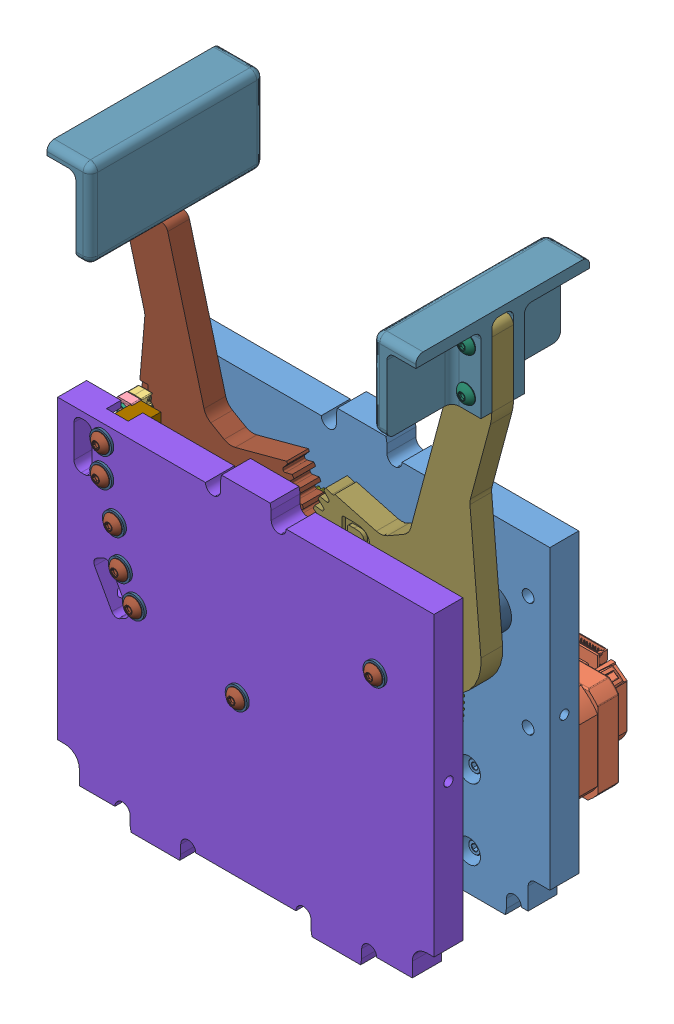
SolidWorks assembly R_ASSY_200_rev3, configuration Default. Lengths in mm. (continued)
Mates (geometry in assembly coordinates): (continued)
- Concentric109: concentric: cylinder of R_203_01_rev4-1 through (-32.103 255.9661 146.893) axis (0 0 1) radius 3.175; cylinder of 91125A453_18-8 SS FEM THRDED ROUND STANDOFF-2 through (-32.103 255.9661 146.893) axis (0 0 -1) radius 3.175
- Width4: width: plane of 91125A453_18-8 SS FEM THRDED ROUND STANDOFF-2 through (-32.103 255.9661 146.893) normal (0 0 1); plane of 91125A453_18-8 SS FEM THRDED ROUND STANDOFF-2 through (-32.103 255.9661 137.368) normal (0 0 -1); plane of R_203_01_rev4-1 through (-14.6848 152.2703 137.368) normal (0 0 -1); plane of R_203_01_rev4-1 through (-14.6848 152.2703 146.893) normal (0 0 1)
- Concentric110: concentric: cylinder of R_203_02_rev4-1 through (117.0334 275.0161 137.368) axis (0 0 -1) radius 3.175; cylinder of 91125A453_18-8 SS FEM THRDED ROUND STANDOFF-4 through (117.0334 275.0161 137.368) axis (0 0 1) radius 3.175
- Width5: width: plane of 91125A453_18-8 SS FEM THRDED ROUND STANDOFF-4 through (117.0334 275.0161 137.368) normal (0 0 -1); plane of 91125A453_18-8 SS FEM THRDED ROUND STANDOFF-4 through (117.0334 275.0161 146.893) normal (0 0 1); plane of R_203_02_rev4-1 through (99.6152 152.2703 146.893) normal (0 0 1); plane of R_203_02_rev4-1 through (99.6152 152.2703 137.368) normal (0 0 -1)
- Concentric111: concentric: cylinder of R_203_02_rev4-1 through (117.0334 255.9661 137.368) axis (0 0 -1) radius 3.175; cylinder of 91125A453_18-8 SS FEM THRDED ROUND STANDOFF-6 through (117.0334 255.9661 137.368) axis (0 0 1) radius 3.175
- Width6: width: plane of 91125A453_18-8 SS FEM THRDED ROUND STANDOFF-6 through (117.0334 255.9661 137.368) normal (0 0 -1); plane of 91125A453_18-8 SS FEM THRDED ROUND STANDOFF-6 through (117.0334 255.9661 146.893) normal (0 0 1); plane of R_203_02_rev4-1 through (99.6152 152.2703 137.368) normal (0 0 -1); plane of R_203_02_rev4-1 through (99.6152 152.2703 146.893) normal (0 0 1)
- Width7: width: plane of R_203_05-1 through (16.7976 249.6161 146.893) normal (0 0 -1); plane of R_203_05-1 through (16.7976 249.6161 137.368) normal (0 0 1); plane of R_203_01_rev4-1 through (-14.6848 152.2703 137.368) normal (0 0 -1); plane of R_203_01_rev4-1 through (-14.6848 152.2703 146.893) normal (0 0 1)
- Concentric112: concentric: cylinder of R_203_01_rev4-1 through (-32.103 275.0161 146.893) axis (0 0 1) radius 3.175; cylinder of R_203_05-1 through (-32.103 275.0161 132.6055) axis (0 0 -1) radius 2.2479
- Concentric113: concentric: cylinder of R_203_01_rev4-1 through (-32.103 255.9661 146.893) axis (0 0 1) radius 3.175; cylinder of R_203_05-1 through (-32.103 255.9661 132.6055) axis (0 0 -1) radius 2.2479
- Concentric114: concentric: cylinder of R_203_05-1 through (-32.103 275.0161 132.6055) axis (0 0 -1) radius 2.2479; cylinder of 92949A192_18-8 SS BUTTON HEAD HEX DRIVE SCREW-19 through (-32.103 275.0161 153.8653) axis (0 0 1) radius 3.9624
- Coincident104: coincident: plane of R_203_05-1 through (18.1551 249.6161 151.6555) normal (0 0 1); plane of 92949A192_18-8 SS BUTTON HEAD HEX DRIVE SCREW-19 through (-31.8728 271.0604 151.6555) normal (0 0 -1)
- Concentric115: concentric: cylinder of R_203_05-1 through (-32.103 255.9661 132.6055) axis (0 0 -1) radius 2.2479; cylinder of 92949A192_18-8 SS BUTTON HEAD HEX DRIVE SCREW-20 through (-32.103 255.9661 153.8653) axis (0 0 1) radius 3.9624
- Coincident105: coincident: plane of R_203_05-1 through (18.1551 249.6161 151.6555) normal (0 0 1); plane of 92949A192_18-8 SS BUTTON HEAD HEX DRIVE SCREW-20 through (-31.2485 252.0969 151.6555) normal (0 0 -1)
- Concentric116: concentric: cylinder of R_203_05-1 through (-32.103 275.0161 132.6055) axis (0 0 -1) radius 2.2479; cylinder of 92949A192_18-8 SS BUTTON HEAD HEX DRIVE SCREW-22 through (-32.103 275.0161 130.3957) axis (0 0 -1) radius 3.9624
- Coincident106: coincident: plane of R_203_05-1 through (18.1551 249.6161 132.6055) normal (0 0 -1); plane of 92949A192_18-8 SS BUTTON HEAD HEX DRIVE SCREW-22 through (-33.0016 271.157 132.6055) normal (0 0 1)
- Concentric118: concentric: cylinder of R_203_05-1 through (-32.103 255.9661 132.6055) axis (0 0 -1) radius 2.2479; cylinder of 92949A192_18-8 SS BUTTON HEAD HEX DRIVE SCREW-25 through (-32.103 255.9661 130.3957) axis (0 0 -1) radius 3.9624
- Coincident112: coincident: plane of R_203_05-1 through (18.1551 249.6161 132.6055) normal (0 0 -1); plane of 92949A192_18-8 SS BUTTON HEAD HEX DRIVE SCREW-25 through (-33.3574 252.2075 132.6055) normal (0 0 1)
- Concentric119: concentric: cylinder of 92949A192_18-8 SS BUTTON HEAD HEX DRIVE SCREW-29 through (117.0334 275.0161 130.3957) axis (0 0 -1) radius 3.9624; cylinder of R_203_05-2 through (117.0334 275.0161 151.6555) axis (0 0 1) radius 2.2479
- Coincident113: coincident: plane of 92949A192_18-8 SS BUTTON HEAD HEX DRIVE SCREW-29 through (117.2636 278.9718 132.6055) normal (0 0 1); plane of R_203_05-2 through (66.7754 249.6161 132.6055) normal (0 0 -1)
- Concentric120: concentric: cylinder of 92949A192_18-8 SS BUTTON HEAD HEX DRIVE SCREW-30 through (117.0334 255.9661 130.3957) axis (0 0 -1) radius 3.9624; cylinder of R_203_05-2 through (117.0334 255.9661 151.6555) axis (0 0 1) radius 2.2479
- Coincident114: coincident: plane of 92949A192_18-8 SS BUTTON HEAD HEX DRIVE SCREW-30 through (117.8879 259.8353 132.6055) normal (0 0 1); plane of R_203_05-2 through (66.7754 249.6161 132.6055) normal (0 0 -1)
- Concentric121: concentric: cylinder of 92949A192_18-8 SS BUTTON HEAD HEX DRIVE SCREW-27 through (117.0334 275.0161 153.8653) axis (0 0 1) radius 3.9624; cylinder of R_203_05-2 through (117.0334 275.0161 151.6555) axis (0 0 1) radius 2.2479
- Coincident115: coincident: plane of 92949A192_18-8 SS BUTTON HEAD HEX DRIVE SCREW-27 through (117.9321 271.157 151.6555) normal (0 0 -1); plane of R_203_05-2 through (66.7754 249.6161 151.6555) normal (0 0 1)
- Concentric122: concentric: cylinder of 92949A192_18-8 SS BUTTON HEAD HEX DRIVE SCREW-28 through (117.0334 255.9661 153.8653) axis (0 0 1) radius 3.9624; cylinder of R_203_05-2 through (117.0334 255.9661 151.6555) axis (0 0 1) radius 2.2479
- Coincident116: coincident: plane of 92949A192_18-8 SS BUTTON HEAD HEX DRIVE SCREW-28 through (118.2879 252.2075 151.6555) normal (0 0 -1); plane of R_203_05-2 through (66.7754 249.6161 151.6555) normal (0 0 1)
- Width8: width: plane of R_203_05-2 through (68.1329 249.6161 137.368) normal (0 0 1); plane of R_203_05-2 through (68.1329 249.6161 146.893) normal (0 0 -1); plane of R_203_02_rev4-1 through (99.6152 152.2703 137.368) normal (0 0 -1); plane of R_203_02_rev4-1 through (99.6152 152.2703 146.893) normal (0 0 1)
- Concentric123: concentric: cylinder of R_203_02_rev4-1 through (117.0334 275.0161 137.368) axis (0 0 -1) radius 3.175; cylinder of R_203_05-2 through (117.0334 275.0161 151.6555) axis (0 0 1) radius 2.2479
- Concentric124: concentric: cylinder of R_203_02_rev4-1 through (117.0334 255.9661 137.368) axis (0 0 -1) radius 3.175; cylinder of R_203_05-2 through (117.0334 255.9661 151.6555) axis (0 0 1) radius 2.2479
- Concentric125: concentric: cylinder of R_200_03_rev2-1 through (39.2022 113.0052 167.5305) axis (0 0 -1) radius 3.175; cylinder of 2797T100_LIGHT DUTY DRY-RUNNING THRUST BEARING-1 through (39.2022 113.0052 124.668) axis (0 0 -1) radius 3.175
- Coincident117: coincident: plane of R_200_01_rev3-1 through (42.4652 115.7578 123.0805) normal (0 0 1); plane of 2797T100_LIGHT DUTY DRY-RUNNING THRUST BEARING-1 through (39.2022 113.0052 123.0805) normal (0 0 -1)
- Concentric126: concentric: cylinder of R_200_05-1 through (39.2022 113.0052 151.6555) axis (0 0 1) radius 4.7625; cylinder of 6338K413_OIL-EMBEDDED FLANGED SLEEVE BEARING-1 through (39.2022 113.0052 137.368) axis (0 0 -1) radius 4.7879
- Coincident118: coincident: plane of R_200_05-1 through (39.2022 113.0052 126.2555) normal (0 0 -1); plane of 6338K413_OIL-EMBEDDED FLANGED SLEEVE BEARING-1 through (39.2022 113.0052 126.2555) normal (0 0 1)
- Concentric127: concentric: cylinder of R_200_05-1 through (39.2022 113.0052 151.6555) axis (0 0 1) radius 4.7625; cylinder of 6338K413_OIL-EMBEDDED FLANGED SLEEVE BEARING-2 through (39.2022 113.0052 140.543) axis (0 0 1) radius 4.7879
- Coincident119: coincident: plane of R_200_05-1 through (37.3814 109.3355 151.6555) normal (0 0 1); plane of 6338K413_OIL-EMBEDDED FLANGED SLEEVE BEARING-2 through (39.2022 113.0052 151.6555) normal (0 0 -1)
- Concentric128: concentric: cylinder of R_200_03_rev2-1 through (39.2022 113.0052 167.5305) axis (0 0 -1) radius 3.175; cylinder of 6338K413_OIL-EMBEDDED FLANGED SLEEVE BEARING-1 through (39.2022 113.0052 137.368) axis (0 0 -1) radius 3.1877
- Coincident120: coincident: plane of 2797T100_LIGHT DUTY DRY-RUNNING THRUST BEARING-1 through (39.2022 113.0052 124.668) normal (0 0 1); plane of 6338K413_OIL-EMBEDDED FLANGED SLEEVE BEARING-1 through (39.2022 113.0052 124.668) normal (0 0 -1)
- Concentric129: concentric: cylinder of R_203_01_rev4-1 through (-14.6848 152.2703 146.893) axis (0 0 1) radius 6.3373; cylinder of 6338K414_OIL-EMBEDDED FLANGED SLEEVE BEARING-1 through (-14.6848 152.2703 142.1305) axis (0 0 -1) radius 6.3627
- Coincident121: coincident: plane of R_203_01_rev4-1 through (-14.6848 152.2703 137.368) normal (0 0 -1); plane of 6338K414_OIL-EMBEDDED FLANGED SLEEVE BEARING-1 through (-14.6848 152.2703 137.368) normal (0 0 1)
- Concentric130: concentric: cylinder of R_203_01_rev4-1 through (-14.6848 152.2703 146.893) axis (0 0 1) radius 6.3373; cylinder of 6338K414_OIL-EMBEDDED FLANGED SLEEVE BEARING-2 through (-14.6848 152.2703 142.1305) axis (0 0 1) radius 6.3627
- Coincident122: coincident: plane of R_203_01_rev4-1 through (-14.6848 152.2703 146.893) normal (0 0 1); plane of 6338K414_OIL-EMBEDDED FLANGED SLEEVE BEARING-2 through (-14.6848 152.2703 146.893) normal (0 0 -1)
- Concentric131: concentric: cylinder of R_203_02_rev4-1 through (99.6152 152.2703 137.368) axis (0 0 -1) radius 6.3373; cylinder of 6338K414_OIL-EMBEDDED FLANGED SLEEVE BEARING-4 through (99.6152 152.2703 142.1305) axis (0 0 1) radius 6.3627
- Coincident123: coincident: plane of R_203_02_rev4-1 through (99.6152 152.2703 146.893) normal (0 0 1); plane of 6338K414_OIL-EMBEDDED FLANGED SLEEVE BEARING-4 through (99.6152 152.2703 146.893) normal (0 0 -1)
- Concentric132: concentric: cylinder of R_203_02_rev4-1 through (99.6152 152.2703 137.368) axis (0 0 -1) radius 6.3373; cylinder of 6338K414_OIL-EMBEDDED FLANGED SLEEVE BEARING-6 through (99.6152 152.2703 142.1305) axis (0 0 -1) radius 6.3627
- Coincident124: coincident: plane of R_203_02_rev4-1 through (99.6152 152.2703 137.368) normal (0 0 -1); plane of 6338K414_OIL-EMBEDDED FLANGED SLEEVE BEARING-6 through (99.6152 152.2703 137.368) normal (0 0 1)
- Concentric133: concentric: cylinder of R_200_04-2 through (99.6152 152.2703 167.5305) axis (0 0 -1) radius 4.7625; cylinder of 6338K414_OIL-EMBEDDED FLANGED SLEEVE BEARING-6 through (99.6152 152.2703 142.1305) axis (0 0 -1) radius 4.7752
- Concentric134: concentric: cylinder of R_200_04-1 through (-14.6848 152.2703 116.7305) axis (0 0 1) radius 4.7625; cylinder of 6338K414_OIL-EMBEDDED FLANGED SLEEVE BEARING-1 through (-14.6848 152.2703 142.1305) axis (0 0 -1) radius 4.7752
- Width9: width: plane of R_200_02_rev3-1 through (42.4652 115.7578 161.1805) normal (0 0 -1); plane of R_200_01_rev3-1 through (42.4652 115.7578 123.0805) normal (0 0 1); plane of 6338K414_OIL-EMBEDDED FLANGED SLEEVE BEARING-4 through (99.6152 152.2703 148.4805) normal (0 0 1); plane of 6338K414_OIL-EMBEDDED FLANGED SLEEVE BEARING-6 through (99.6152 152.2703 135.7805) normal (0 0 -1)
- Concentric135: concentric: cylinder of R_200_04-2 through (99.6152 152.2703 167.5305) axis (0 0 -1) radius 4.7625; cylinder of R_200_09_SPCR_rev3-5 through (99.6152 152.2703 148.4805) axis (0 0 1) radius 4.8895
- Coincident125: coincident: plane of 6338K414_OIL-EMBEDDED FLANGED SLEEVE BEARING-4 through (99.6152 152.2703 148.4805) normal (0 0 1); plane of R_200_09_SPCR_rev3-5 through (99.6152 152.2703 148.4805) normal (0 0 -1)
- Concentric136: concentric: cylinder of R_200_04-1 through (-14.6848 152.2703 116.7305) axis (0 0 1) radius 4.7625; cylinder of R_200_09_SPCR_rev3-7 through (-14.6848 152.2703 148.4805) axis (0 0 1) radius 4.8895
- Coincident126: coincident: plane of 6338K414_OIL-EMBEDDED FLANGED SLEEVE BEARING-2 through (-14.6848 152.2703 148.4805) normal (0 0 1); plane of R_200_09_SPCR_rev3-7 through (-14.6848 152.2703 148.4805) normal (0 0 -1)
- Width10: width: plane of R_200_02_rev3-1 through (42.4652 115.7578 161.1805) normal (0 0 -1); plane of R_200_01_rev3-1 through (42.4652 115.7578 123.0805) normal (0 0 1); plane of 6338K414_OIL-EMBEDDED FLANGED SLEEVE BEARING-1 through (-14.6848 152.2703 135.7805) normal (0 0 -1); plane of 6338K414_OIL-EMBEDDED FLANGED SLEEVE BEARING-2 through (-14.6848 152.2703 148.4805) normal (0 0 1)
- Concentric137: concentric: cylinder of R_200_01_rev3-1 through (89.5331 85.2143 123.0805) axis (0 0 1) radius 1.7; cylinder of 91116A120_TYPE 18-8 STAINLESS STL OVERSIZED FLAT WASHER-12 through (89.5331 85.2143 117.6305) axis (0 0 -1) radius 1.6
- Coincident127: coincident: plane of R_200_01_rev3-1 through (89.5331 85.2143 116.7305) normal (0 0 1); plane of 91116A120_TYPE 18-8 STAINLESS STL OVERSIZED FLAT WASHER-12 through (89.5331 85.2143 116.7305) normal (0 0 -1)
- Coincident128: coincident: plane of 91116A120_TYPE 18-8 STAINLESS STL OVERSIZED FLAT WASHER-12 through (89.5331 85.2143 117.6305) normal (0 0 1); plane of 91292A027_TYPE 18-8 SS SOCKET HEAD CAP SCREW-1 through (89.5331 85.2143 117.6305) normal (0 0 -1)
- Concentric138: concentric: cylinder of 91116A120_TYPE 18-8 STAINLESS STL OVERSIZED FLAT WASHER-12 through (89.5331 85.2143 117.6305) axis (0 0 -1) radius 1.6; cylinder of 91292A027_TYPE 18-8 SS SOCKET HEAD CAP SCREW-1 through (89.5331 85.2143 120.6305) axis (0 0 -1) radius 2.75
- Concentric141: concentric: cylinder of dc1c-a1aa-1/dc1c-a1aa_03-1 through (-27.4348 169.2553 154.8305) axis (1 0 0) radius 1.15; cylinder of 92095A104_BUTTON HEAD HEX DRIVE SCREW-1 through (-31.5598 169.2553 154.8305) axis (-1 0 0) radius 1.9
- Coincident133: coincident: plane of dc1c-a1aa-1/dc1c-a1aa_03-1 through (-30.6598 169.2553 154.8305) normal (-1 0 0); plane of 92095A104_BUTTON HEAD HEX DRIVE SCREW-1 through (-30.6598 167.3553 154.8305) normal (1 0 0)
- Coincident134: coincident: plane of R_200_02_rev3-1 through (42.4652 115.7578 167.5305) normal (0 0 -1); plane of R_200_10-2 through (-20.241 174.0203 167.5305) normal (0 0 1)
- Concentric142: concentric: cylinder of R_200_02_rev3-1 through (-20.241 180.3703 167.5305) axis (0 0 -1) radius 2.2479; cylinder of R_200_10-2 through (-20.241 180.3703 167.5305) axis (0 0 1) radius 1.7272
- Concentric143: concentric: cylinder of R_200_02_rev3-1 through (-20.241 167.6703 167.5305) axis (0 0 -1) radius 2.2479; cylinder of R_200_10-2 through (-20.241 167.6703 167.5305) axis (0 0 1) radius 1.7272
- Coincident136: coincident: plane of dc1c-a1aa-1/dc1c-a1aa_03-1 through (-24.2098 169.2553 154.8305) normal (1 0 0); plane of R_200_10-2 through (-24.2098 164.4953 153.243) normal (-1 0 0)
- Concentric144: concentric: cylinder of dc1c-a1aa-1/dc1c-a1aa_03-1 through (-27.4348 169.2553 154.8305) axis (1 0 0) radius 1.15; cylinder of R_200_10-2 through (-24.2098 169.2553 154.8305) axis (-1 0 0) radius 0.8
- Slot1: slot: cylinder of dc1c-a1aa-1/dc1c-a1aa_03-1 through (-27.4348 178.9053 154.8305) axis (1 0 0) radius 1.15; cylinder of R_200_10-2 through (-24.2098 178.7853 154.8305) axis (-1 0 0) radius 0.8; cylinder of dc1c-a1aa-1/dc1c-a1aa_03-1 through (-27.4348 178.6653 154.8305) axis (1 0 0) radius 1.15
- Concentric145: concentric: cylinder of R_200_10-2 through (-24.2098 178.7853 154.8305) axis (-1 0 0) radius 0.8; cylinder of 92095A104_BUTTON HEAD HEX DRIVE SCREW-2 through (-31.5598 178.7853 154.8305) axis (-1 0 0) radius 1.9
- Coincident137: coincident: plane of dc1c-a1aa-1/dc1c-a1aa_03-1 through (-30.6598 169.2553 154.8305) normal (-1 0 0); plane of 92095A104_BUTTON HEAD HEX DRIVE SCREW-2 through (-30.6598 179.1152 152.9593) normal (1 0 0)
- Coincident139: coincident: plane of R_200_02_rev3-1 through (42.4652 115.7578 167.5305) normal (0 0 -1); plane of R_200_10-3 through (-8.9998 130.5536 167.5305) normal (0 0 1)
- Concentric146: concentric: cylinder of R_200_02_rev3-1 through (-12.0783 136.1074 167.5305) axis (0 0 -1) radius 2.2479; cylinder of R_200_10-3 through (-12.0783 136.1074 167.5305) axis (0 0 1) radius 1.7272
- Concentric148: concentric: cylinder of R_200_02_rev3-1 through (-5.9212 124.9998 167.5305) axis (0 0 -1) radius 2.2479; cylinder of R_200_10-3 through (-5.9212 124.9998 167.5305) axis (0 0 1) radius 1.7272
- Coincident140: coincident: plane of R_200_10-3 through (-7.8531 120.2988 153.243) normal (-0.87462 -0.48481 0); plane of dc1c-a1aa-2/dc1c-a1aa_03-1 through (-14.781 132.7971 154.8305) normal (0.87462 0.48481 0)
- Concentric149: concentric: cylinder of R_200_10-3 through (-14.781 132.7971 154.8305) axis (-0.87462 -0.48481 0) radius 0.8; cylinder of ? through (-17.6017 131.2336 154.8305) axis (-0.87462 -0.48481 0) radius 1.15
- Slot2: slot: cylinder of ? through (-12.9233 122.7935 154.8305) axis (-0.87462 -0.48481 0) radius 1.15; cylinder of R_200_10-3 through (-10.1608 124.462 154.8305) axis (-0.87462 -0.48481 0) radius 0.8; cylinder of ? through (-13.0396 123.0034 154.8305) axis (-0.87462 -0.48481 0) radius 1.15
- Concentric150: concentric: cylinder of ? through (-17.6017 131.2336 154.8305) axis (-0.87462 -0.48481 0) radius 1.15; cylinder of 92095A104_BUTTON HEAD HEX DRIVE SCREW-3 through (-21.2095 129.2337 154.8305) axis (-0.87462 -0.48481 0) radius 1.9
- Coincident141: coincident: plane of ? through (-20.4223 129.6701 154.8305) normal (-0.87462 -0.48481 0); plane of 92095A104_BUTTON HEAD HEX DRIVE SCREW-3 through (-19.7733 128.4992 156.1787) normal (0.87462 0.48481 0)
- Concentric151: concentric: cylinder of R_200_10-3 through (-10.1608 124.462 154.8305) axis (-0.87462 -0.48481 0) radius 0.8; cylinder of 92095A104_BUTTON HEAD HEX DRIVE SCREW-5 through (-16.5893 120.8986 154.8305) axis (-0.87462 -0.48481 0) radius 1.9
- Coincident142: coincident: plane of ? through (-20.4223 129.6701 154.8305) normal (-0.87462 -0.48481 0); plane of 92095A104_BUTTON HEAD HEX DRIVE SCREW-5 through (-16.1456 121.9546 156.5934) normal (0.87462 0.48481 0)
- Concentric153: concentric: cylinder of R_200_01_rev3-1 through (4.3652 69.7203 116.7305) axis (0 0 1) radius 11.0754; cylinder of STP-MTR-17048E-2 through (4.3652 69.7203 110.3805) axis (0 0 1) radius 10.9982
- Concentric154: concentric: cylinder of R_200_01_rev3-1 through (74.0391 69.7203 116.7305) axis (0 0 1) radius 11.0754; cylinder of STP-MTR-17048E-1 through (74.0391 69.7203 110.3805) axis (0 0 1) radius 10.9982
- Coincident143: coincident: plane of R_200_02_rev3-1 through (42.4652 115.7578 173.8805) normal (0 0 1); plane of 92141A009_TYPE 18-8 STAINLESS STEEL FLAT WASHER-5 through (-20.241 180.3703 173.8805) normal (0 0 -1)
- Concentric155: concentric: cylinder of R_200_02_rev3-1 through (-20.241 180.3703 167.5305) axis (0 0 -1) radius 2.2479; cylinder of 92141A009_TYPE 18-8 STAINLESS STEEL FLAT WASHER-5 through (-20.241 180.3703 174.8965) axis (0 0 -1) radius 2.1844
- Coincident144: coincident: plane of 92141A009_TYPE 18-8 STAINLESS STEEL FLAT WASHER-5 through (-20.241 180.3703 174.8965) normal (0 0 1); plane of 92949A194_18-8 SS BUTTON HEAD HEX DRIVE SCREW-12 through (-19.821 184.3104 174.8965) normal (0 0 -1)
- Concentric156: concentric: cylinder of 92141A009_TYPE 18-8 STAINLESS STEEL FLAT WASHER-5 through (-20.241 180.3703 174.8965) axis (0 0 -1) radius 2.1844; cylinder of 92949A194_18-8 SS BUTTON HEAD HEX DRIVE SCREW-12 through (-20.241 180.3703 177.1063) axis (0 0 1) radius 3.9624
- Coincident145: coincident: plane of 92141A009_TYPE 18-8 STAINLESS STEEL FLAT WASHER-6 through (-20.241 167.6703 174.8965) normal (0 0 1); plane of 92949A194_18-8 SS BUTTON HEAD HEX DRIVE SCREW-17 through (-19.2016 171.494 174.8965) normal (0 0 -1)
- Concentric157: concentric: cylinder of 92141A009_TYPE 18-8 STAINLESS STEEL FLAT WASHER-6 through (-20.241 167.6703 174.8965) axis (0 0 -1) radius 2.1844; cylinder of 92949A194_18-8 SS BUTTON HEAD HEX DRIVE SCREW-17 through (-20.241 167.6703 177.1063) axis (0 0 1) radius 3.9624
- Coincident146: coincident: plane of R_200_02_rev3-1 through (42.4652 115.7578 173.8805) normal (0 0 1); plane of 92141A009_TYPE 18-8 STAINLESS STEEL FLAT WASHER-6 through (-20.241 167.6703 173.8805) normal (0 0 -1)
- Concentric158: concentric: cylinder of R_200_02_rev3-1 through (-20.241 167.6703 167.5305) axis (0 0 -1) radius 2.2479; cylinder of 92141A009_TYPE 18-8 STAINLESS STEEL FLAT WASHER-6 through (-20.241 167.6703 174.8965) axis (0 0 -1) radius 2.1844
- Coincident147: coincident: plane of 92141A009_TYPE 18-8 STAINLESS STEEL FLAT WASHER-7 through (-14.6848 152.2703 174.8965) normal (0 0 1); plane of 92949A194_18-8 SS BUTTON HEAD HEX DRIVE SCREW-18 through (-13.167 155.9305 174.8965) normal (0 0 -1)
- Concentric159: concentric: cylinder of 92141A009_TYPE 18-8 STAINLESS STEEL FLAT WASHER-7 through (-14.6848 152.2703 174.8965) axis (0 0 -1) radius 2.1844; cylinder of 92949A194_18-8 SS BUTTON HEAD HEX DRIVE SCREW-18 through (-14.6848 152.2703 177.1063) axis (0 0 1) radius 3.9624
- Coincident148: coincident: plane of R_200_02_rev3-1 through (42.4652 115.7578 173.8805) normal (0 0 1); plane of 92141A009_TYPE 18-8 STAINLESS STEEL FLAT WASHER-7 through (-14.6848 152.2703 173.8805) normal (0 0 -1)
- Concentric160: concentric: cylinder of R_200_02_rev3-1 through (-14.6848 152.2703 161.1805) axis (0 0 -1) radius 2.2479; cylinder of 92141A009_TYPE 18-8 STAINLESS STEEL FLAT WASHER-7 through (-14.6848 152.2703 174.8965) axis (0 0 -1) radius 2.1844
- Coincident149: coincident: plane of 92141A009_TYPE 18-8 STAINLESS STEEL FLAT WASHER-8 through (-12.0783 136.1074 174.8965) normal (0 0 1); plane of 92949A194_18-8 SS BUTTON HEAD HEX DRIVE SCREW-19 through (-10.2259 139.6102 174.8965) normal (0 0 -1)
- Concentric161: concentric: cylinder of 92141A009_TYPE 18-8 STAINLESS STEEL FLAT WASHER-8 through (-12.0783 136.1074 174.8965) axis (0 0 -1) radius 2.1844; cylinder of 92949A194_18-8 SS BUTTON HEAD HEX DRIVE SCREW-19 through (-12.0783 136.1074 177.1063) axis (0 0 1) radius 3.9624
- Coincident150: coincident: plane of R_200_02_rev3-1 through (42.4652 115.7578 173.8805) normal (0 0 1); plane of 92141A009_TYPE 18-8 STAINLESS STEEL FLAT WASHER-8 through (-12.0783 136.1074 173.8805) normal (0 0 -1)
- Concentric162: concentric: cylinder of R_200_02_rev3-1 through (-12.0783 136.1074 167.5305) axis (0 0 -1) radius 2.2479; cylinder of 92141A009_TYPE 18-8 STAINLESS STEEL FLAT WASHER-8 through (-12.0783 136.1074 174.8965) axis (0 0 -1) radius 2.1844
- Coincident151: coincident: plane of 92141A009_TYPE 18-8 STAINLESS STEEL FLAT WASHER-9 through (-5.9212 124.9998 174.8965) normal (0 0 1); plane of 92949A194_18-8 SS BUTTON HEAD HEX DRIVE SCREW-20 through (-3.8809 128.3965 174.8965) normal (0 0 -1)
- Concentric163: concentric: cylinder of 92141A009_TYPE 18-8 STAINLESS STEEL FLAT WASHER-9 through (-5.9212 124.9998 174.8965) axis (0 0 -1) radius 2.1844; cylinder of 92949A194_18-8 SS BUTTON HEAD HEX DRIVE SCREW-20 through (-5.9212 124.9998 177.1063) axis (0 0 1) radius 3.9624
- Coincident152: coincident: plane of R_200_02_rev3-1 through (42.4652 115.7578 173.8805) normal (0 0 1); plane of 92141A009_TYPE 18-8 STAINLESS STEEL FLAT WASHER-9 through (-5.9212 124.9998 173.8805) normal (0 0 -1)
- Concentric164: concentric: cylinder of R_200_02_rev3-1 through (-5.9212 124.9998 167.5305) axis (0 0 -1) radius 2.2479; cylinder of 92141A009_TYPE 18-8 STAINLESS STEEL FLAT WASHER-9 through (-5.9212 124.9998 174.8965) axis (0 0 -1) radius 2.1844
- Coincident153: coincident: plane of 92141A009_TYPE 18-8 STAINLESS STEEL FLAT WASHER-10 through (39.2022 113.0052 174.8965) normal (0 0 1); plane of 92949A194_18-8 SS BUTTON HEAD HEX DRIVE SCREW-16 through (41.2754 116.3819 174.8965) normal (0 0 -1)
- Concentric165: concentric: cylinder of 92141A009_TYPE 18-8 STAINLESS STEEL FLAT WASHER-10 through (39.2022 113.0052 174.8965) axis (0 0 -1) radius 2.1844; cylinder of 92949A194_18-8 SS BUTTON HEAD HEX DRIVE SCREW-16 through (39.2022 113.0052 177.1063) axis (0 0 1) radius 3.9624
- Coincident154: coincident: plane of R_200_02_rev3-1 through (42.4652 115.7578 173.8805) normal (0 0 1); plane of 92141A009_TYPE 18-8 STAINLESS STEEL FLAT WASHER-10 through (39.2022 113.0052 173.8805) normal (0 0 -1)
- Concentric166: concentric: cylinder of R_200_02_rev3-1 through (39.2022 113.0052 161.1805) axis (0 0 -1) radius 2.2479; cylinder of 92141A009_TYPE 18-8 STAINLESS STEEL FLAT WASHER-10 through (39.2022 113.0052 174.8965) axis (0 0 -1) radius 2.1844
- Coincident155: coincident: plane of 92141A009_TYPE 18-8 STAINLESS STEEL FLAT WASHER-11 through (99.6152 152.2703 174.8965) normal (0 0 1); plane of 92949A194_18-8 SS BUTTON HEAD HEX DRIVE SCREW-11 through (101.5492 155.7287 174.8965) normal (0 0 -1)
- Concentric167: concentric: cylinder of 92141A009_TYPE 18-8 STAINLESS STEEL FLAT WASHER-11 through (99.6152 152.2703 174.8965) axis (0 0 -1) radius 2.1844; cylinder of 92949A194_18-8 SS BUTTON HEAD HEX DRIVE SCREW-11 through (99.6152 152.2703 177.1063) axis (0 0 1) radius 3.9624
- Coincident156: coincident: plane of R_200_02_rev3-1 through (42.4652 115.7578 173.8805) normal (0 0 1); plane of 92141A009_TYPE 18-8 STAINLESS STEEL FLAT WASHER-11 through (99.6152 152.2703 173.8805) normal (0 0 -1)
- Concentric168: concentric: cylinder of R_200_02_rev3-1 through (99.6152 152.2703 161.1805) axis (0 0 -1) radius 2.2479; cylinder of 92141A009_TYPE 18-8 STAINLESS STEEL FLAT WASHER-11 through (99.6152 152.2703 174.8965) axis (0 0 -1) radius 2.1844
- Coincident162: coincident: plane of 92141A009_TYPE 18-8 STAINLESS STEEL FLAT WASHER-14 through (-14.6848 152.2703 109.3645) normal (0 0 -1); plane of 92949A194_18-8 SS BUTTON HEAD HEX DRIVE SCREW-22 through (-10.8775 153.3681 109.3645) normal (0 0 1)
- Concentric171: concentric: cylinder of 92141A009_TYPE 18-8 STAINLESS STEEL FLAT WASHER-14 through (-14.6848 152.2703 109.3645) axis (0 0 1) radius 2.1844; cylinder of 92949A194_18-8 SS BUTTON HEAD HEX DRIVE SCREW-22 through (-14.6848 152.2703 107.1547) axis (0 0 -1) radius 3.9624
- Coincident163: coincident: plane of R_200_01_rev3-1 through (42.4652 115.7578 110.3805) normal (0 0 -1); plane of 92141A009_TYPE 18-8 STAINLESS STEEL FLAT WASHER-14 through (-14.6848 152.2703 110.3805) normal (0 0 1)
- Concentric172: concentric: cylinder of R_200_01_rev3-1 through (-14.6848 152.2703 123.0805) axis (0 0 1) radius 2.2479; cylinder of 92141A009_TYPE 18-8 STAINLESS STEEL FLAT WASHER-14 through (-14.6848 152.2703 109.3645) axis (0 0 1) radius 2.1844
- Coincident165: coincident: plane of 92141A009_TYPE 18-8 STAINLESS STEEL FLAT WASHER-16 through (39.2022 113.0052 109.3645) normal (0 0 -1); plane of 92949A194_18-8 SS BUTTON HEAD HEX DRIVE SCREW-24 through (42.761 114.7474 109.3645) normal (0 0 1)
- Concentric174: concentric: cylinder of 92141A009_TYPE 18-8 STAINLESS STEEL FLAT WASHER-16 through (39.2022 113.0052 109.3645) axis (0 0 1) radius 2.1844; cylinder of 92949A194_18-8 SS BUTTON HEAD HEX DRIVE SCREW-24 through (39.2022 113.0052 107.1547) axis (0 0 -1) radius 3.9624
- Coincident166: coincident: plane of R_200_01_rev3-1 through (42.4652 115.7578 110.3805) normal (0 0 -1); plane of 92141A009_TYPE 18-8 STAINLESS STEEL FLAT WASHER-16 through (39.2022 113.0052 110.3805) normal (0 0 1)
- Concentric175: concentric: cylinder of R_200_01_rev3-1 through (39.2022 113.0052 123.0805) axis (0 0 1) radius 2.2479; cylinder of 92141A009_TYPE 18-8 STAINLESS STEEL FLAT WASHER-16 through (39.2022 113.0052 109.3645) axis (0 0 1) radius 2.1844
- Coincident168: coincident: plane of 92141A009_TYPE 18-8 STAINLESS STEEL FLAT WASHER-18 through (99.6152 152.2703 109.3645) normal (0 0 -1); plane of 92949A194_18-8 SS BUTTON HEAD HEX DRIVE SCREW-26 through (102.8174 154.6041 109.3645) normal (0 0 1)
- Concentric177: concentric: cylinder of 92141A009_TYPE 18-8 STAINLESS STEEL FLAT WASHER-18 through (99.6152 152.2703 109.3645) axis (0 0 1) radius 2.1844; cylinder of 92949A194_18-8 SS BUTTON HEAD HEX DRIVE SCREW-26 through (99.6152 152.2703 107.1547) axis (0 0 -1) radius 3.9624
- Coincident169: coincident: plane of R_200_01_rev3-1 through (42.4652 115.7578 110.3805) normal (0 0 -1); plane of 92141A009_TYPE 18-8 STAINLESS STEEL FLAT WASHER-18 through (99.6152 152.2703 110.3805) normal (0 0 1)
- Concentric178: concentric: cylinder of R_200_01_rev3-1 through (99.6152 152.2703 123.0805) axis (0 0 1) radius 2.2479; cylinder of 92141A009_TYPE 18-8 STAINLESS STEEL FLAT WASHER-18 through (99.6152 152.2703 109.3645) axis (0 0 1) radius 2.1844
- Coincident170: coincident: plane of R_200_01_rev3-1 through (42.4652 115.7578 110.3805) normal (0 0 -1); plane of 93365A142_HEAT-SET INSERTS FOR PLASTICS-1 through (115.4902 114.0178 110.3805) normal (0 0 -1)
- Concentric180: concentric: cylinder of R_200_01_rev3-1 through (115.4902 114.0178 110.3805) axis (0 0 -1) radius 2.6098; cylinder of 93365A142_HEAT-SET INSERTS FOR PLASTICS-1 through (115.4902 114.0178 110.3805) axis (0 0 -1) radius 2.7051
- Coincident171: coincident: plane of R_200_01_rev3-1 through (42.4652 115.7578 110.3805) normal (0 0 -1); plane of 93365A142_HEAT-SET INSERTS FOR PLASTICS-4 through (115.4902 164.0178 110.3805) normal (0 0 -1)
- Concentric181: concentric: cylinder of R_200_01_rev3-1 through (115.4902 164.0178 110.3805) axis (0 0 -1) radius 2.6098; cylinder of 93365A142_HEAT-SET INSERTS FOR PLASTICS-4 through (115.4902 164.0178 110.3805) axis (0 0 -1) radius 2.7051
- Coincident172: coincident: plane of R_200_01_rev3-1 through (42.4652 115.7578 110.3805) normal (0 0 -1); plane of 93365A142_HEAT-SET INSERTS FOR PLASTICS-3 through (-30.5598 164.0178 110.3805) normal (0 0 -1)
- Concentric182: concentric: cylinder of R_200_01_rev3-1 through (-30.5598 164.0178 110.3805) axis (0 0 -1) radius 2.6098; cylinder of 93365A142_HEAT-SET INSERTS FOR PLASTICS-3 through (-30.5598 164.0178 110.3805) axis (0 0 -1) radius 2.7051
- Coincident173: coincident: plane of R_200_01_rev3-1 through (42.4652 115.7578 110.3805) normal (0 0 -1); plane of 93365A142_HEAT-SET INSERTS FOR PLASTICS-2 through (-30.5598 114.0178 110.3805) normal (0 0 -1)
- Concentric183: concentric: cylinder of R_200_01_rev3-1 through (-30.5598 114.0178 110.3805) axis (0 0 -1) radius 2.6098; cylinder of 93365A142_HEAT-SET INSERTS FOR PLASTICS-2 through (-30.5598 114.0178 110.3805) axis (0 0 -1) radius 2.7051
